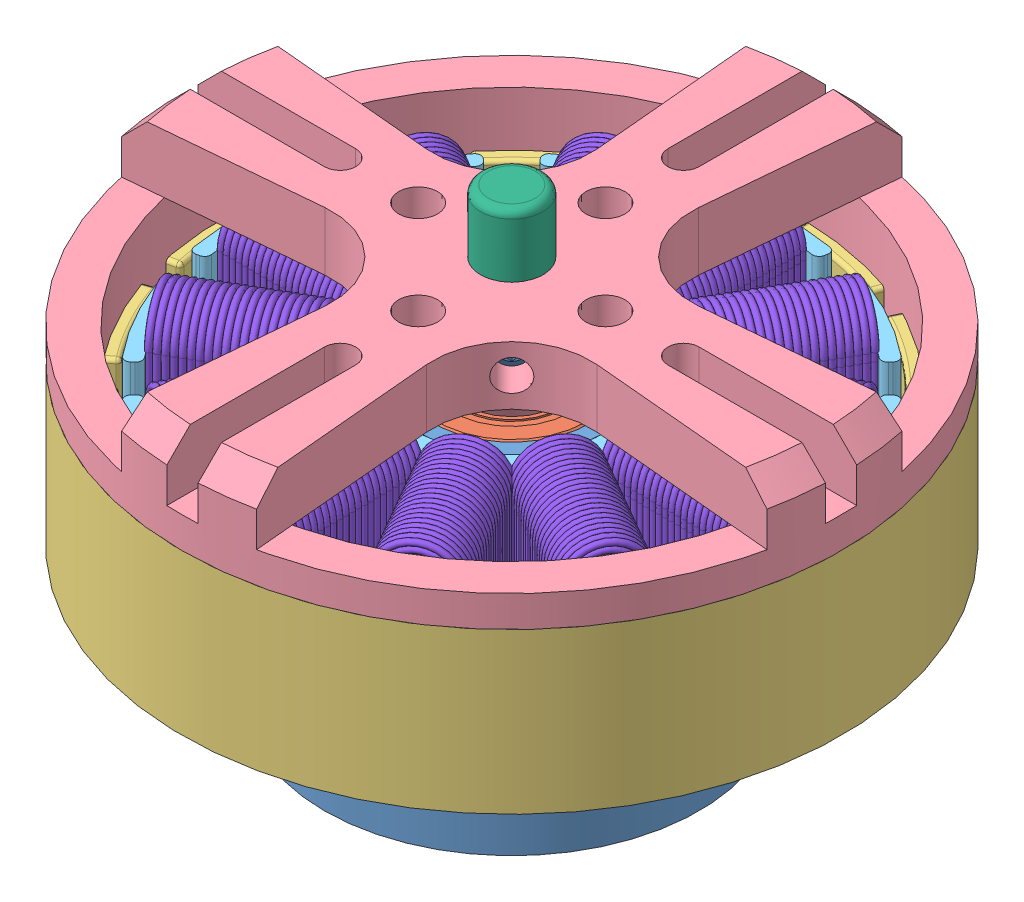
SolidWorks assembly D4215 Brushless Motor, configuration Default. Lengths in mm.
Overall size (51.98 30.25 51.98).
11 component instances, 10 part files, 26 mates.
Components (placement in the parent):
- D4215 Stator Base-1: D4215 Stator Base [Default] at (12.4338 7.3776 20.085) size (24 18 24)
- 7804K1_Stainless Steel Ball Bearing-1: 7804K1_Stainless Steel Ball Bearing [7804K1] at (12.4338 9.3776 20.085) x (1 0 0) z (0 -1 0) size (10 10 4)
- 7804K1_Stainless Steel Ball Bearing-2: 7804K1_Stainless Steel Ball Bearing [7804K1] at (12.4338 23.3776 20.085) x (1 0 0) z (0 -1 0) size (10 10 4)
- D4215 Magnet ring-1: D4215 Magnet ring [Default] at (12.4338 16.1276 20.085) x (0.963873 0 -0.266363) z (0.266363 0 0.963873) size (42.25 10.25 42.25)
- D4215 Rotor Top-1: D4215 Rotor Top [Default] at (12.4338 26.3776 20.085) x (0 0 -1) z (0 1 0) size (42.25 42.25 8.75)
- D4215 Stator-1: D4215 Stator [Default] at (12.4338 16.3776 20.085) x (1 0 0) z (0 1 0) size (35.45 35.45 9)
- D4215 Shaft-1: D4215 Shaft [Default] at (12.4338 5.8776 20.085) x (0.707107 0 -0.707107) z (0.707107 0 0.707107) size (4 30.25 4)
- 98541A112_BLACK-FINISH STEEL EXTERNAL RETAINING RING-1: 98541A112_BLACK-FINISH STEEL EXTERNAL RETAINING RING [98541A112] at (12.4338 6.9276 20.085) x (0 1 0) z (0.355569 0 0.93465) size (0.4 6.8 5.16)
- D4215 Stator coils-1: D4215 Stator coils [Default] at (12.4338 25.3776 20.085) x (1 0 0) z (0 1 0) size (33.33 33.33 13.72)
- Brass washer-1: Brass washer [91635A370] at (12.4338 7.3776 20.085) x (0.999983 0 0.00588) z (0 -1 0) size (5.5 5.5 0.25)
- 91390A094_ALLOY STEEL CUP POINT SET SCREW-1: 91390A094_ALLOY STEEL CUP POINT SET SCREW [91390A094] at (14.7006 30.2526 22.3518) x (0.707107 0 -0.707107) z (0.707107 0 0.707107) size (2.61 2.89 3.45)
Mates (geometry in assembly coordinates):
- Concentric1: concentric aligned: cylinder of D4215 Stator Base-1 through (12.4338 7.3776 20.085) axis (0 -1 0) radius 5; cylinder of 7804K1_Stainless Steel Ball Bearing-1 through (12.4338 7.3776 20.085) axis (0 -1 0) radius 5
- Coincident1: coincident anti-aligned: plane of D4215 Stator Base-1 through (7.4338 11.3776 20.085) normal (0 -1 0); plane of 7804K1_Stainless Steel Ball Bearing-1 through (12.4338 11.3776 24.885) normal (0 1 0)
- Coincident2: coincident anti-aligned: plane of D4215 Stator Base-1 through (7.9338 21.3776 20.085) normal (0 1 0); plane of 7804K1_Stainless Steel Ball Bearing-2 through (12.4338 21.3776 24.885) normal (0 -1 0)
- Concentric2: concentric aligned: cylinder of D4215 Stator Base-1 through (12.4338 7.3776 20.085) axis (0 -1 0) radius 5; cylinder of 7804K1_Stainless Steel Ball Bearing-2 through (12.4338 21.3776 20.085) axis (0 -1 0) radius 5
- Concentric3: concentric aligned: cylinder of D4215 Stator Base-1 through (12.4338 7.3776 20.085) axis (0 -1 0) radius 6; cylinder of D4215 Magnet ring-1 through (12.4338 16.1276 20.085) axis (0 -1 0) radius 21.125
- Concentric4: concentric aligned: cylinder of D4215 Magnet ring-1 through (12.4338 16.1276 20.085) axis (0 -1 0) radius 21.125; cylinder of D4215 Rotor Top-1 through (12.4338 32.1276 20.085) axis (0 -1 0) radius 21.125
- Coincident3: coincident anti-aligned: plane of D4215 Magnet ring-1 through (-6.675 26.3776 25.3656) normal (0 1 0); plane of D4215 Rotor Top-1 through (12.4338 26.3776 20.085) normal (0 -1 0)
- Coincident4: coincident anti-aligned: plane of 7804K1_Stainless Steel Ball Bearing-2 through (12.4338 25.3776 22.285) normal (0 1 0); plane of D4215 Rotor Top-1 through (9.4338 25.3776 20.085) normal (0 -1 0)
- InPlace1: in place: plane of D4215 Stator Base-1 through (4.4338 17.3776 20.085) normal (0 1 0); plane of ? through (0 17.3776 0) normal (0 1 0); moOrthogonalPlaneRef_w of D4215 Stator Base-1 through (4.4338 17.3776 20.085) normal (0 1 0); plane of ? through (0 17.3776 0) normal (0 0 -1); plane of D4215 Stator Base-1 through (4.4338 17.3776 20.085) normal (0 1 0); plane of ? through (0 17.3776 0) normal (1 0 0); plane of D4215 Stator Base-1 through (5.6838 16.3776 20.085) normal (0 1 0); unknown of D4215 Stator-1
- Coincident5: coincident aligned: plane of D4215 Stator Base-1; plane of D4215 Stator-1
- Coincident6: coincident aligned: moOrthogonalPlaneRef_w of D4215 Stator Base-1 through (12.4338 16.3776 20.085) normal (0 0 -1); plane of D4215 Stator-1 through (12.4338 16.3776 20.085) normal (0 0 -1)
- Coincident7: coincident anti-aligned: moOrthogonalPlaneRef_w of D4215 Stator Base-1 through (12.4338 16.3776 20.085) normal (-1 0 0); plane of D4215 Stator-1 through (12.4338 16.3776 20.085) normal (1 0 0)
- Concentric5: concentric aligned: cylinder of D4215 Rotor Top-1 through (12.4338 32.1276 20.085) axis (0 -1 0) radius 2; cylinder of D4215 Shaft-1 through (12.4338 5.8776 20.085) axis (0 -1 0) radius 2
- Distance1: distance = 4 mm aligned: plane of D4215 Shaft-1 through (12.4338 36.1276 20.085) normal (0 1 0); plane of D4215 Rotor Top-1 through (12.4338 32.1276 20.085) normal (0 1 0)
- Coincident9: coincident anti-aligned: plane of 98541A112_BLACK-FINISH STEEL EXTERNAL RETAINING RING-1 through (12.4338 7.1276 20.085) normal (0 1 0); plane of D4215 Shaft-1 through (12.4338 7.1276 20.085) normal (0 -1 0)
- Concentric6: concentric aligned: cylinder of D4215 Shaft-1 through (12.4338 5.8776 20.085) axis (0 -1 0) radius 1.5; cylinder of 98541A112_BLACK-FINISH STEEL EXTERNAL RETAINING RING-1 through (12.4338 7.1276 20.085) axis (0 -1 0) radius 1.85
- InPlace2: in place: plane of ? through (6.4338 25.3776 20.085) normal (0 1 0); plane of ? through (0 25.3776 0) normal (0 1 0); plane of ? through (6.4338 25.3776 20.085) normal (0 1 0); plane of ? through (0 25.3776 0) normal (0 0 -1); plane of ? through (6.4338 25.3776 20.085) normal (0 1 0); plane of ? through (0 25.3776 0) normal (1 0 0); plane of D4215 Stator-1 through (7.4338 25.3776 20.085) normal (0 1 0); unknown of D4215 Stator coils-1
- Coincident10: coincident aligned: plane of D4215 Stator-1; plane of D4215 Stator coils-1
- Coincident11: coincident aligned: moOrthogonalPlaneRef_w of D4215 Stator-1 through (12.4338 25.3776 20.085) normal (0 0 -1); plane of D4215 Stator coils-1 through (12.4338 25.3776 20.085) normal (0 0 -1)
- Coincident12: coincident anti-aligned: moOrthogonalPlaneRef_w of D4215 Stator-1 through (12.4338 25.3776 20.085) normal (-1 0 0); plane of D4215 Stator coils-1 through (12.4338 25.3776 20.085) normal (1 0 0)
- Coincident13: coincident anti-aligned: plane of 7804K1_Stainless Steel Ball Bearing-1 through (12.4338 7.3776 23.3212) normal (0 -1 0); plane of 91635A370_BRASS FLAT WASHER-1 through (12.4338 7.3776 20.085) normal (0 1 0)
- Concentric7: concentric anti-aligned: cylinder of D4215 Shaft-1 through (12.4338 5.8776 20.085) axis (0 -1 0) radius 2; cylinder of 91635A370_BRASS FLAT WASHER-1 through (12.4338 7.1276 20.085) axis (0 1 0) radius 2
- Parallel1: parallel anti-aligned: plane of D4215 Rotor Top-1 through (12.4338 26.3776 20.085) normal (-0.707107 0 -0.707107); plane of D4215 Shaft-1 through (13.4945 5.8776 21.1456) normal (0.707107 0 0.707107)
- Concentric8: concentric anti-aligned: cylinder of D4215 Rotor Top-1 through (33.5588 30.2526 41.21) axis (-0.707107 0 -0.707107) radius 1; circle of 91390A094_ALLOY STEEL CUP POINT SET SCREW-1
- Coincident15: coincident aligned: plane of D4215 Shaft-1 through (13.4945 5.8776 21.1456) normal (0.707107 0 0.707107); circle of 91390A094_ALLOY STEEL CUP POINT SET SCREW-1
- Perpendicular1: perpendicular: plane of assembly through (0 0 0) normal (0 0 1); plane of D4215 Rotor Top-1 through (11.4338 1.7028 20.085) normal (1 0 0)
